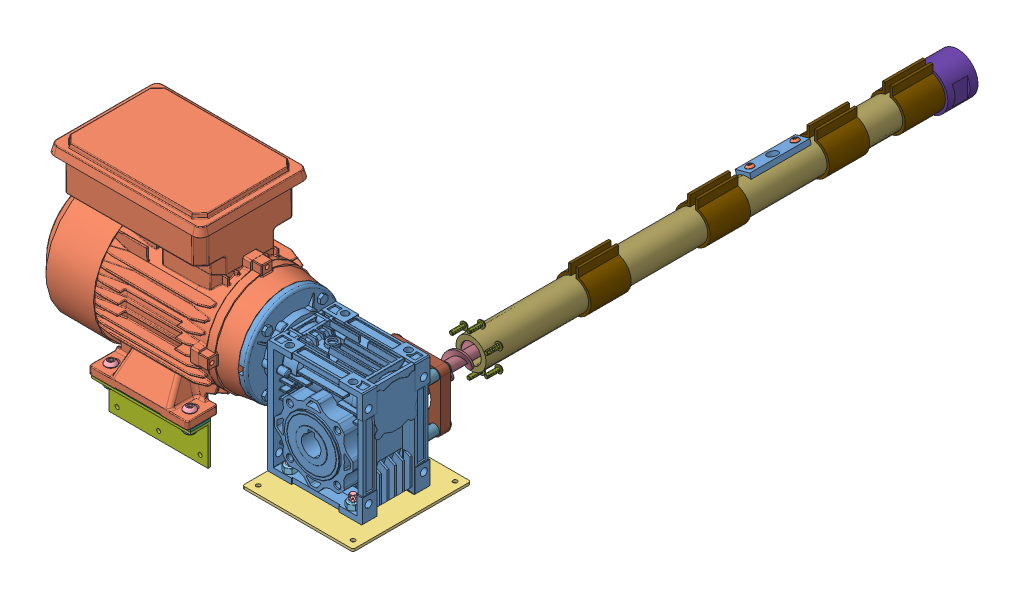
SolidWorks assembly coplete extruder assembly, configuration Default. Lengths in mm.
Overall size (405 416.05 925.2).
61 component instances, 24 part files, 64 mates.
Components (placement in the parent):
- motor assembly-1: motor assembly [Default] at (94.2301 96.5097 233.5212) size (405 416.05 596.46)
  - Redüktör Limöz LRP 50 1e25-1: Redüktör Limöz LRP 50 1e25 [Varsayılan] at (76.2256 70.7411 124.7447) size (140 170.5 120)
  - Gamak 0.75 KW Monofeze Motor-1: Gamak 0.75 KW Monofeze Motor [Varsayılan] at (-3.7744 121.2411 124.7447) x (0 0 1) z (-1 0 0) size (161.7 221.7 280.5)
  - gearbox plate-2: gearbox plate [Default] at (86.2256 7.5661 124.7447) x (0 0 -1) z (1 0 0) size (149 3.17 140)
  - 91239A427_CLASS 10.9 STL BUTTON-HEAD SOCKET CAP SCREW-1: 91239A427_CLASS 10.9 STL BUTTON-HEAD SOCKET CAP SCREW [91239A427] at (36.7256 3.1661 159.7447) x (1 0 0) z (0 -1 0) size (14 14 30.18)
  - 91239A427_CLASS 10.9 STL BUTTON-HEAD SOCKET CAP SCREW-2: 91239A427_CLASS 10.9 STL BUTTON-HEAD SOCKET CAP SCREW [91239A427] at (36.7256 3.1661 89.7447) x (1 0 0) z (0 -1 0) size (14 14 30.18)
  - 91239A427_CLASS 10.9 STL BUTTON-HEAD SOCKET CAP SCREW-3: 91239A427_CLASS 10.9 STL BUTTON-HEAD SOCKET CAP SCREW [91239A427] at (116.7256 3.1661 89.7447) x (1 0 0) z (0 -1 0) size (14 14 30.18)
  - 91239A427_CLASS 10.9 STL BUTTON-HEAD SOCKET CAP SCREW-4: 91239A427_CLASS 10.9 STL BUTTON-HEAD SOCKET CAP SCREW [91239A427] at (116.7256 3.1661 159.7447) x (1 0 0) z (0 -1 0) size (14 14 30.18)
  - 94645A210_ZINC-PLATED CLASS 10 STL NYLON-INSERT LOCKNUT-1: 94645A210_ZINC-PLATED CLASS 10 STL NYLON-INSERT LOCKNUT [94645A210] at (36.7256 17.7411 159.7447) size (13 8.23 15.01)
  - 94645A210_ZINC-PLATED CLASS 10 STL NYLON-INSERT LOCKNUT-2: 94645A210_ZINC-PLATED CLASS 10 STL NYLON-INSERT LOCKNUT [94645A210] at (116.7256 17.7411 159.7447) size (13 8.23 15.01)
  - 94645A210_ZINC-PLATED CLASS 10 STL NYLON-INSERT LOCKNUT-3: 94645A210_ZINC-PLATED CLASS 10 STL NYLON-INSERT LOCKNUT [94645A210] at (116.7256 17.7411 89.7447) size (13 8.23 15.01)
  - 94645A210_ZINC-PLATED CLASS 10 STL NYLON-INSERT LOCKNUT-4: 94645A210_ZINC-PLATED CLASS 10 STL NYLON-INSERT LOCKNUT [94645A210] at (36.7256 17.7411 89.7447) size (13 8.23 15.01)
  - 91239A427_CLASS 10.9 STL BUTTON-HEAD SOCKET CAP SCREW-5: 91239A427_CLASS 10.9 STL BUTTON-HEAD SOCKET CAP SCREW [91239A427] at (-159.7744 55.6411 189.7447) x (1 0 0) z (0 1 0) size (14 14 30.18)
  - 91239A427_CLASS 10.9 STL BUTTON-HEAD SOCKET CAP SCREW-6: 91239A427_CLASS 10.9 STL BUTTON-HEAD SOCKET CAP SCREW [91239A427] at (-59.7744 55.6411 189.7447) x (1 0 0) z (0 1 0) size (14 14 30.18)
  - 91239A427_CLASS 10.9 STL BUTTON-HEAD SOCKET CAP SCREW-7: 91239A427_CLASS 10.9 STL BUTTON-HEAD SOCKET CAP SCREW [91239A427] at (-159.7744 55.6411 59.6704) x (1 0 0) z (0 1 0) size (14 14 30.18)
  - 91239A427_CLASS 10.9 STL BUTTON-HEAD SOCKET CAP SCREW-8: 91239A427_CLASS 10.9 STL BUTTON-HEAD SOCKET CAP SCREW [91239A427] at (-59.7744 55.6411 59.7447) x (1 0 0) z (0 1 0) size (14 14 30.18)
  - motor dampener-1: motor dampener [Default] at (-109.7744 38.3661 188.7697) size (125 2.88 25.4)
  - motor mount-1: motor mount [Default] at (-172.2744 -12.4339 176.0697) x (0 0 -1) z (1 0 0) size (25.4 50.8 125)
  - motor mount-2: motor mount [Default] at (-47.2744 -12.4339 73.3454) x (0 0 1) z (-1 0 0) size (25.4 50.8 125)
  - motor dampener-3: motor dampener [Default] at (-109.7744 38.3661 60.6454) x (-1 0 0) z (0 0 -1) size (125 2.88 25.4)
  - 94645A210_ZINC-PLATED CLASS 10 STL NYLON-INSERT LOCKNUT-5: 94645A210_ZINC-PLATED CLASS 10 STL NYLON-INSERT LOCKNUT [94645A210] at (-159.7744 35.1911 189.7447) x (-0.837169 0 -0.546944) z (-0.546944 0 0.837169) size (13 8.23 15.01)
  - 94645A210_ZINC-PLATED CLASS 10 STL NYLON-INSERT LOCKNUT-6: 94645A210_ZINC-PLATED CLASS 10 STL NYLON-INSERT LOCKNUT [94645A210] at (-59.7744 35.1911 189.7447) x (-0.837169 0 -0.546944) z (-0.546944 0 0.837169) size (13 8.23 15.01)
  - 94645A210_ZINC-PLATED CLASS 10 STL NYLON-INSERT LOCKNUT-7: 94645A210_ZINC-PLATED CLASS 10 STL NYLON-INSERT LOCKNUT [94645A210] at (-159.7744 35.1911 59.6704) x (-0.837169 0 -0.546944) z (-0.546944 0 0.837169) size (13 8.23 15.01)
  - 94645A210_ZINC-PLATED CLASS 10 STL NYLON-INSERT LOCKNUT-8: 94645A210_ZINC-PLATED CLASS 10 STL NYLON-INSERT LOCKNUT [94645A210] at (-59.7744 35.1911 59.6704) x (-0.837169 0 -0.546944) z (-0.546944 0 0.837169) size (13 8.23 15.01)
- motor keyed assembly-1: motor keyed assembly [Default] at (179.7303 160.2957 356.7051) x (-1 0 0) z (0 0 -1) size (38.35 38.35 70)
  - key-1: key [Default] at (9.2746 18.9552 8.4391) size (8 7 32)
  - motor adaptor-1: motor adaptor [Default] at (9.2746 6.9552 4.4391) size (31.75 31.75 70)
  - 92095A208_18-8 SS BUTTON-HEAD SOCKET CAP SCREW-1: 92095A208_18-8 SS BUTTON-HEAD SOCKET CAP SCREW [92095A208] at (9.2746 29.2556 61.7391) x (0.982212 0 -0.187776) z (0 1 0) size (9.5 9.5 13.21)
  - 92095A208_18-8 SS BUTTON-HEAD SOCKET CAP SCREW-2: 92095A208_18-8 SS BUTTON-HEAD SOCKET CAP SCREW [92095A208] at (31.575 6.9552 61.7391) x (0 -0.452478 -0.891775) z (1 0 0) size (9.5 9.5 13.21)
- hopper body-1: hopper body [Default] at (130.4149 128.2753 188.7593) size (75 75 12.7)
  - hopper body-1: hopper body [Default] at (40.0409 38.9756 14.8067) (suppressed, hidden)
  - thrust bearing plate-1: thrust bearing plate [Default] at (40.0409 38.9756 78.3067) size (75 75 12.7)
- barrel Assembly-1: barrel Assembly [Default] at (387.3105 -120.5193 393.6593) x (-1 0 0) z (0 0 -1) size (38.1 38.1 609.6)
  - barrel-1: barrel [Default] at (216.8548 287.7701 113.8933) size (38.1 38.1 609.6)
  - pelletizer plate mount-1: pelletizer plate mount [Default] at (216.8548 287.7701 190.0933) (suppressed, hidden)
- 2_1 compression degas screw-1: 2_1 compression degas screw [Default] at (170.4557 167.2509 -378.134) size (26.05 26.04 688.01)
- thrust bering plate stsandoff-1: thrust bering plate stsandoff [Default] at (140.4557 197.2509 279.766) size (12.7 12.7 35)
- thrust bering plate stsandoff-2: thrust bering plate stsandoff [Default] at (140.4557 137.2509 279.766) size (12.7 12.7 35)
- thrust bering plate stsandoff-3: thrust bering plate stsandoff [Default] at (200.4557 197.2509 279.766) size (12.7 12.7 35)
- thrust bering plate stsandoff-4: thrust bering plate stsandoff [Default] at (200.4557 137.2509 279.766) size (12.7 12.7 35)
- feed tube assembly-1: feed tube assembly [Default] at (151.3893 181.3032 202.7167)
  - hopper tube-1: hopper tube [Default] at (19.0664 1.1876 38.8858) (suppressed, hidden)
  - tube hopper base-1: tube hopper base [Default] at (19.0664 1.1876 38.8858) (suppressed, hidden)
- 92095A299_18-8 SS BUTTON-HEAD SOCKET CAP SCREW-1: 92095A299_18-8 SS BUTTON-HEAD SOCKET CAP SCREW [92095A299] at (200.4557 197.2509 262.666) x (-0.923728 -0.383049 0) z (0 0 -1) size (14 14 60.2)
- 92095A299_18-8 SS BUTTON-HEAD SOCKET CAP SCREW-2: 92095A299_18-8 SS BUTTON-HEAD SOCKET CAP SCREW [92095A299] at (140.4557 197.2509 262.666) x (-0.923728 -0.383049 0) z (0 0 -1) size (14 14 60.2)
- 92095A299_18-8 SS BUTTON-HEAD SOCKET CAP SCREW-3: 92095A299_18-8 SS BUTTON-HEAD SOCKET CAP SCREW [92095A299] at (140.4557 137.2509 262.666) x (-0.923728 -0.383049 0) z (0 0 -1) size (14 14 60.2)
- 92095A299_18-8 SS BUTTON-HEAD SOCKET CAP SCREW-4: 92095A299_18-8 SS BUTTON-HEAD SOCKET CAP SCREW [92095A299] at (200.4557 137.2509 262.666) x (-0.923728 -0.383049 0) z (0 0 -1) size (14 14 60.2)
- 92095A212_18-8 SS BUTTON-HEAD SOCKET CAP SCREW-1: 92095A212_18-8 SS BUTTON-HEAD SOCKET CAP SCREW [92095A212] at (170.4557 141.8509 188.116) x (-0.923728 -0.383049 0) z (0 0 -1) size (9.5 9.5 19.24)
- 92095A212_18-8 SS BUTTON-HEAD SOCKET CAP SCREW-2: 92095A212_18-8 SS BUTTON-HEAD SOCKET CAP SCREW [92095A212] at (192.4528 154.5509 188.116) x (-0.923728 -0.383049 0) z (0 0 -1) size (9.5 9.5 19.24)
- 92095A212_18-8 SS BUTTON-HEAD SOCKET CAP SCREW-3: 92095A212_18-8 SS BUTTON-HEAD SOCKET CAP SCREW [92095A212] at (192.4528 179.9509 188.116) x (-0.923728 -0.383049 0) z (0 0 -1) size (9.5 9.5 19.24)
- 92095A212_18-8 SS BUTTON-HEAD SOCKET CAP SCREW-4: 92095A212_18-8 SS BUTTON-HEAD SOCKET CAP SCREW [92095A212] at (170.4557 192.6509 188.116) x (-0.923728 -0.383049 0) z (0 0 -1) size (9.5 9.5 19.24)
- 92095A212_18-8 SS BUTTON-HEAD SOCKET CAP SCREW-5: 92095A212_18-8 SS BUTTON-HEAD SOCKET CAP SCREW [92095A212] at (148.4587 179.9509 188.116) x (-0.923728 -0.383049 0) z (0 0 -1) size (9.5 9.5 19.24)
- 92095A212_18-8 SS BUTTON-HEAD SOCKET CAP SCREW-6: 92095A212_18-8 SS BUTTON-HEAD SOCKET CAP SCREW [92095A212] at (148.4587 154.5509 188.116) x (-0.923728 -0.383049 0) z (0 0 -1) size (9.5 9.5 19.24)
- nozzle-1: nozzle [Default] at (170.4557 167.2509 -374.284) x (0 -1 0) z (0 0 -1) size (50.8 50.8 38.1)
- heater band standing-1: heater band standing [Default] at (170.4557 167.2509 -374.284) size (44.45 53.98 50.8)
- heater band standing-2: heater band standing [Default] at (170.4557 167.2509 -278.484) size (44.45 53.98 50.8)
- heater band standing-3: heater band standing [Default] at (170.4557 167.2509 -127.684) size (44.45 53.98 50.8)
- heater band standing-4: heater band standing [Default] at (170.4557 167.2509 23.116) size (44.45 53.98 50.8)
- degas body base-1: degas body base [Default] at (166.1826 183.1983 -183.784) x (0 0 -1) z (0.965926 0.258819 0) size (76.07 6.35 19)
- 91239A222_CLASS 10.9 STL BUTTON-HEAD SOCKET CAP SCREW-1: 91239A222_CLASS 10.9 STL BUTTON-HEAD SOCKET CAP SCREW [91239A222] at (163.8274 191.9882 -155.209) x (0.933013 0.25 0.258819) z (-0.258819 0.965926 0) size (9.5 9.5 11.19)
- 91239A222_CLASS 10.9 STL BUTTON-HEAD SOCKET CAP SCREW-2: 91239A222_CLASS 10.9 STL BUTTON-HEAD SOCKET CAP SCREW [91239A222] at (163.8274 191.9882 -212.359) x (0.933013 0.25 0.258819) z (-0.258819 0.965926 0) size (9.5 9.5 11.19)
Mates (geometry in assembly coordinates):
- Coincident1: coincident anti-aligned: plane of motor assembly-1/Redüktör Limöz LRP 50 1e25-1 through (170.4557 167.2509 312.266) normal (0 0 -1); plane of motor keyed assembly-1/motor adaptor-1 through (170.4557 167.2509 312.266) normal (0 0 1)
- Parallel1: parallel anti-aligned: plane of motor assembly-1/Redüktör Limöz LRP 50 1e25-1 through (174.4557 179.0936 288.766) normal (-1 0 0); plane of motor keyed assembly-1/key-1 through (174.4557 175.7509 316.266) normal (1 0 0)
- Concentric1: concentric aligned: cylinder of motor assembly-1/Redüktör Limöz LRP 50 1e25-1 through (170.4557 167.2509 288.766) axis (0 0 1) radius 12.5; cylinder of motor keyed assembly-1/motor adaptor-1 through (170.4557 167.2509 282.266) axis (0 0 1) radius 15.875
- Concentric2: concentric aligned: cylinder of motor keyed assembly-1/motor adaptor-1 through (170.4557 167.2509 307.666) axis (0 0 -1) radius 9.5504; cylinder of hopper body-1/hopper body-1 through (170.4557 167.2509 279.766) axis (0 0 -1) radius 12.7254
- Parallel2: parallel aligned: plane of motor assembly-1/gearbox plate-2 through (180.4557 107.2509 358.266) normal (0 1 0); plane of hopper body-1/hopper body-1 through (170.4557 182.4909 203.566) normal (0 1 0)
- Coincident4: coincident anti-aligned: plane of hopper body-1/hopper body-1 through (170.4557 167.2509 203.566) normal (0 0 -1); plane of barrel Assembly-1/pelletizer plate mount-1 through (170.4557 167.2509 203.566) normal (0 0 1)
- Concentric3: concentric aligned: cylinder of hopper body-1/hopper body-1 through (170.4557 192.6509 209.916) axis (0 0 -1) radius 2.665; cylinder of barrel Assembly-1/pelletizer plate mount-1 through (170.4557 192.6509 203.567) axis (0 0 -1) radius 2.665
- Concentric4: concentric anti-aligned: cylinder of hopper body-1/hopper body-1 through (170.4557 167.2509 216.266) axis (0 0 -1) radius 31.75; cylinder of barrel Assembly-1/pelletizer plate mount-1 through (170.4557 167.2509 190.866) axis (0 0 1) radius 31.75
- Concentric5: concentric aligned: cylinder of hopper body-1/hopper body-1 through (170.4557 167.2509 279.766) axis (0 0 -1) radius 12.7254; cylinder of 2_1 compression degas screw-1 through (170.4557 167.2509 282.266) axis (0 0 -1) radius 12.7
- Parallel3: parallel aligned: plane of motor keyed assembly-1/92095A208_18-8 SS BUTTON-HEAD SOCKET CAP SCREW-1 through (169.9863 189.5513 292.5105) normal (0 1 0); plane of 2_1 compression degas screw-1 through (170.4557 174.8709 288.616) normal (0 1 0)
- Coincident7: coincident anti-aligned: plane of motor assembly-1/Redüktör Limöz LRP 50 1e25-1 through (170.4557 167.2509 314.766) normal (0 0 -1); plane of thrust bering plate stsandoff-4 through (200.4557 137.2509 314.766) normal (0 0 1)
- Concentric6: concentric anti-aligned: cylinder of motor assembly-1/Redüktör Limöz LRP 50 1e25-1 through (200.4557 137.2509 314.766) axis (0 0 1) radius 3.5; cylinder of thrust bering plate stsandoff-4 through (200.4557 137.2509 314.766) axis (0 0 -1) radius 4.165
- Coincident8: coincident anti-aligned: plane of hopper body-1/thrust bearing plate-1 through (170.4557 167.2509 279.766) normal (0 0 1); plane of thrust bering plate stsandoff-4 through (200.4557 137.2509 279.766) normal (0 0 -1)
- Coincident9: coincident anti-aligned: circle of motor keyed assembly-1/motor adaptor-1; plane of 2_1 compression degas screw-1 through (170.4557 167.2509 307.666) normal (0 0 1)
- Coincident10: coincident anti-aligned: plane of motor assembly-1/Redüktör Limöz LRP 50 1e25-1 through (170.4557 167.2509 314.766) normal (0 0 -1); plane of thrust bering plate stsandoff-3 through (200.4557 197.2509 314.766) normal (0 0 1)
- Concentric7: concentric anti-aligned: cylinder of motor assembly-1/Redüktör Limöz LRP 50 1e25-1 through (200.4557 197.2509 314.766) axis (0 0 1) radius 3.5; cylinder of thrust bering plate stsandoff-3 through (200.4557 197.2509 314.766) axis (0 0 -1) radius 6.35
- Coincident11: coincident anti-aligned: plane of hopper body-1/thrust bearing plate-1 through (170.4557 167.2509 279.766) normal (0 0 1); plane of thrust bering plate stsandoff-1 through (140.4557 197.2509 279.766) normal (0 0 -1)
- Concentric8: concentric anti-aligned: cylinder of hopper body-1/thrust bearing plate-1 through (140.4557 197.2509 267.065) axis (0 0 1) radius 4.165; cylinder of thrust bering plate stsandoff-1 through (140.4557 197.2509 314.766) axis (0 0 -1) radius 6.35
- Coincident12: coincident anti-aligned: plane of hopper body-1/thrust bearing plate-1 through (170.4557 167.2509 279.766) normal (0 0 1); plane of thrust bering plate stsandoff-2 through (140.4557 137.2509 279.766) normal (0 0 -1)
- Concentric9: concentric anti-aligned: cylinder of hopper body-1/thrust bearing plate-1 through (140.4557 137.2509 267.065) axis (0 0 1) radius 4.165; cylinder of thrust bering plate stsandoff-2 through (140.4557 137.2509 314.766) axis (0 0 -1) radius 6.35
- Coincident13: coincident anti-aligned: plane of hopper body-1/hopper body-1 through (170.4557 182.4909 203.566) normal (0 1 0); plane of feed tube assembly-1/tube hopper base-1 through (170.4557 182.4909 241.6025) normal (0 -1 0)
- Concentric10: concentric aligned: cylinder of hopper body-1/hopper body-1 through (185.7757 176.1409 221.266) axis (0 1 0) radius 2.5; cylinder of feed tube assembly-1/tube hopper base-1 through (185.7757 182.4899 221.266) axis (0 1 0) radius 2.665
- Concentric11: concentric aligned: cylinder of hopper body-1/hopper body-1 through (155.1357 176.1409 221.266) axis (0 1 0) radius 2.5; cylinder of feed tube assembly-1/tube hopper base-1 through (155.1357 182.4899 221.266) axis (0 1 0) radius 2.665
- Coincident14: coincident anti-aligned: plane of hopper body-1/thrust bearing plate-1 through (170.4557 167.2509 267.066) normal (0 0 -1); plane of 92095A299_18-8 SS BUTTON-HEAD SOCKET CAP SCREW-4 through (203.1371 130.7848 267.066) normal (0 0 1)
- Concentric12: concentric anti-aligned: cylinder of hopper body-1/thrust bearing plate-1 through (200.4557 137.2509 267.065) axis (0 0 1) radius 4.165; cylinder of 92095A299_18-8 SS BUTTON-HEAD SOCKET CAP SCREW-4 through (200.4557 137.2509 262.666) axis (0 0 -1) radius 7
- Coincident15: coincident anti-aligned: plane of hopper body-1/thrust bearing plate-1 through (170.4557 167.2509 267.066) normal (0 0 -1); plane of 92095A299_18-8 SS BUTTON-HEAD SOCKET CAP SCREW-1 through (203.1371 190.7848 267.066) normal (0 0 1)
- Concentric13: concentric anti-aligned: cylinder of hopper body-1/thrust bearing plate-1 through (200.4557 197.2509 267.065) axis (0 0 1) radius 4.165; cylinder of 92095A299_18-8 SS BUTTON-HEAD SOCKET CAP SCREW-1 through (200.4557 197.2509 262.666) axis (0 0 -1) radius 7
- Coincident16: coincident anti-aligned: plane of hopper body-1/thrust bearing plate-1 through (170.4557 167.2509 267.066) normal (0 0 -1); plane of 92095A299_18-8 SS BUTTON-HEAD SOCKET CAP SCREW-2 through (143.1371 190.7848 267.066) normal (0 0 1)
- Concentric14: concentric anti-aligned: cylinder of hopper body-1/thrust bearing plate-1 through (140.4557 197.2509 267.065) axis (0 0 1) radius 4.165; cylinder of 92095A299_18-8 SS BUTTON-HEAD SOCKET CAP SCREW-2 through (140.4557 197.2509 262.666) axis (0 0 -1) radius 7
- Coincident17: coincident anti-aligned: plane of hopper body-1/thrust bearing plate-1 through (170.4557 167.2509 267.066) normal (0 0 -1); plane of 92095A299_18-8 SS BUTTON-HEAD SOCKET CAP SCREW-3 through (143.1371 130.7848 267.066) normal (0 0 1)
- Concentric15: concentric anti-aligned: cylinder of hopper body-1/thrust bearing plate-1 through (140.4557 137.2509 267.065) axis (0 0 1) radius 4.165; cylinder of 92095A299_18-8 SS BUTTON-HEAD SOCKET CAP SCREW-3 through (140.4557 137.2509 262.666) axis (0 0 -1) radius 7
- Coincident18: coincident anti-aligned: plane of barrel Assembly-1/pelletizer plate mount-1 through (170.4557 167.2509 190.866) normal (0 0 -1); plane of 92095A212_18-8 SS BUTTON-HEAD SOCKET CAP SCREW-1 through (172.2752 137.4632 190.866) normal (0 0 1)
- Concentric16: concentric aligned: cylinder of barrel Assembly-1/pelletizer plate mount-1 through (170.4557 141.8509 203.567) axis (0 0 -1) radius 2.665; circle of 92095A212_18-8 SS BUTTON-HEAD SOCKET CAP SCREW-1
- Coincident19: coincident anti-aligned: plane of barrel Assembly-1/pelletizer plate mount-1 through (170.4557 167.2509 190.866) normal (0 0 -1); plane of 92095A212_18-8 SS BUTTON-HEAD SOCKET CAP SCREW-2 through (194.2722 150.1632 190.866) normal (0 0 1)
- Concentric17: concentric aligned: cylinder of barrel Assembly-1/pelletizer plate mount-1 through (192.4528 154.5509 203.567) axis (0 0 -1) radius 2.665; cylinder of 92095A212_18-8 SS BUTTON-HEAD SOCKET CAP SCREW-2 through (192.4528 154.5509 188.116) axis (0 0 -1) radius 4.75
- Coincident20: coincident anti-aligned: plane of barrel Assembly-1/pelletizer plate mount-1 through (170.4557 167.2509 190.866) normal (0 0 -1); plane of 92095A212_18-8 SS BUTTON-HEAD SOCKET CAP SCREW-3 through (194.2722 175.5632 190.866) normal (0 0 1)
- Concentric18: concentric aligned: cylinder of barrel Assembly-1/pelletizer plate mount-1 through (192.4528 179.9509 203.567) axis (0 0 -1) radius 2.665; cylinder of 92095A212_18-8 SS BUTTON-HEAD SOCKET CAP SCREW-3 through (192.4528 179.9509 188.116) axis (0 0 -1) radius 4.75
- Coincident21: coincident anti-aligned: plane of barrel Assembly-1/pelletizer plate mount-1 through (170.4557 167.2509 190.866) normal (0 0 -1); plane of 92095A212_18-8 SS BUTTON-HEAD SOCKET CAP SCREW-4 through (172.2752 188.2632 190.866) normal (0 0 1)
- Concentric19: concentric aligned: cylinder of barrel Assembly-1/pelletizer plate mount-1 through (170.4557 192.6509 203.567) axis (0 0 -1) radius 2.665; cylinder of 92095A212_18-8 SS BUTTON-HEAD SOCKET CAP SCREW-4 through (170.4557 192.6509 188.116) axis (0 0 -1) radius 4.75
- Coincident22: coincident anti-aligned: plane of barrel Assembly-1/pelletizer plate mount-1 through (170.4557 167.2509 190.866) normal (0 0 -1); plane of 92095A212_18-8 SS BUTTON-HEAD SOCKET CAP SCREW-5 through (150.2782 175.5632 190.866) normal (0 0 1)
- Concentric20: concentric aligned: cylinder of barrel Assembly-1/pelletizer plate mount-1 through (148.4587 179.9509 203.567) axis (0 0 -1) radius 2.665; cylinder of 92095A212_18-8 SS BUTTON-HEAD SOCKET CAP SCREW-5 through (148.4587 179.9509 188.116) axis (0 0 -1) radius 4.75
- Coincident23: coincident anti-aligned: plane of barrel Assembly-1/pelletizer plate mount-1 through (170.4557 167.2509 190.866) normal (0 0 -1); plane of 92095A212_18-8 SS BUTTON-HEAD SOCKET CAP SCREW-6 through (150.2782 150.1632 190.866) normal (0 0 1)
- Concentric21: concentric aligned: cylinder of barrel Assembly-1/pelletizer plate mount-1 through (148.4587 154.5509 203.567) axis (0 0 -1) radius 2.665; cylinder of 92095A212_18-8 SS BUTTON-HEAD SOCKET CAP SCREW-6 through (148.4587 154.5509 188.116) axis (0 0 -1) radius 4.75
- Coincident24: coincident anti-aligned: plane of barrel Assembly-1/barrel-1 through (170.4557 167.2509 -406.034) normal (0 0 -1); plane of nozzle-1 through (170.4557 167.2509 -406.034) normal (0 0 1)
- Concentric23: concentric aligned: cylinder of barrel Assembly-1/barrel-1 through (170.4557 167.2509 -406.034) axis (0 0 1) radius 19.05; cylinder of nozzle-1 through (170.4557 167.2509 -412.384) axis (0 0 1) radius 25.4
- Concentric24: concentric anti-aligned: cylinder of barrel Assembly-1/barrel-1 through (170.4557 167.2509 -406.034) axis (0 0 1) radius 19.05; cylinder of heater band standing-1 through (170.4557 167.2509 -323.484) axis (0 0 -1) radius 19.05
- Coincident26: coincident anti-aligned: plane of nozzle-1 through (170.4557 167.2509 -374.284) normal (0 0 1); plane of heater band standing-1 through (170.4557 167.2509 -374.284) normal (0 0 -1)
- Parallel5: parallel aligned: plane of nozzle-1 through (192.5537 141.8499 -383.174) normal (1 0 0); plane of heater band standing-1 through (176.8057 199.0009 -323.484) normal (1 0 0)
- Concentric25: concentric anti-aligned: cylinder of barrel Assembly-1/barrel-1 through (170.4557 167.2509 -406.034) axis (0 0 1) radius 19.05; cylinder of heater band standing-2 through (170.4557 167.2509 -227.684) axis (0 0 -1) radius 19.05
- Coincident28: coincident aligned: plane of heater band standing-1 through (176.8057 199.0009 -323.484) normal (1 0 0); plane of heater band standing-2 through (176.8057 199.0009 -227.684) normal (1 0 0)
- Distance1: distance = 45 mm anti-aligned: plane of heater band standing-2 through (170.4557 167.2509 -278.484) normal (0 0 -1); plane of heater band standing-1 through (170.4557 167.2509 -323.484) normal (0 0 1)
- Concentric26: concentric anti-aligned: cylinder of barrel Assembly-1/barrel-1 through (170.4557 167.2509 -406.034) axis (0 0 1) radius 19.05; cylinder of heater band standing-3 through (170.4557 167.2509 -76.884) axis (0 0 -1) radius 19.05
- Distance2: distance = 100 mm anti-aligned: plane of heater band standing-3 through (170.4557 167.2509 -127.684) normal (0 0 -1); plane of heater band standing-2 through (170.4557 167.2509 -227.684) normal (0 0 1)
- Concentric27: concentric anti-aligned: cylinder of barrel Assembly-1/barrel-1 through (170.4557 167.2509 -406.034) axis (0 0 1) radius 19.05; cylinder of heater band standing-4 through (170.4557 167.2509 73.916) axis (0 0 -1) radius 19.05
- Coincident31: coincident aligned: plane of heater band standing-2 through (176.8057 199.0009 -227.684) normal (1 0 0); plane of heater band standing-3 through (176.8057 199.0009 -76.884) normal (1 0 0)
- Coincident32: coincident aligned: plane of heater band standing-3 through (176.8057 199.0009 -76.884) normal (1 0 0); plane of heater band standing-4 through (176.8057 199.0009 73.916) normal (1 0 0)
- Distance3: distance = 100 mm: line of heater band standing-4 through (173.6307 199.0009 23.116) axis (0 -1 0); plane of heater band standing-3 through (170.4557 167.2509 -76.884) normal (0 0 1)
- Coincident34: coincident anti-aligned: plane of barrel Assembly-1/barrel-1 through (166.1826 183.1983 279.766) normal (-0.258819 0.965926 0); plane of degas body base-1 through (166.1826 183.1983 -183.784) normal (0.258819 -0.965926 0)
- Concentric28: concentric aligned: cylinder of barrel Assembly-1/barrel-1 through (166.1826 183.1983 -155.209) axis (-0.258819 0.965926 0) radius 2.1; cylinder of degas body base-1 through (166.1829 183.1973 -155.209) axis (-0.258819 0.965926 0) radius 2.665
- Concentric29: concentric aligned: cylinder of barrel Assembly-1/barrel-1 through (166.1826 183.1983 -212.359) axis (-0.258819 0.965926 0) radius 2.1; cylinder of degas body base-1 through (166.1829 183.1973 -212.359) axis (-0.258819 0.965926 0) radius 2.665
- Coincident35: coincident anti-aligned: plane of degas body base-1 through (164.5391 189.3319 -183.784) normal (-0.258819 0.965926 0); plane of 91239A222_CLASS 10.9 STL BUTTON-HEAD SOCKET CAP SCREW-1 through (163.3516 189.0137 -150.6209) normal (0.258819 -0.965926 0)
- Concentric30: concentric aligned: cylinder of degas body base-1 through (166.1829 183.1973 -155.209) axis (-0.258819 0.965926 0) radius 2.665; cylinder of 91239A222_CLASS 10.9 STL BUTTON-HEAD SOCKET CAP SCREW-1 through (163.8274 191.9882 -155.209) axis (-0.258819 0.965926 0) radius 4.75
- Coincident36: coincident anti-aligned: plane of degas body base-1 through (164.5391 189.3319 -183.784) normal (-0.258819 0.965926 0); plane of 91239A222_CLASS 10.9 STL BUTTON-HEAD SOCKET CAP SCREW-2 through (163.3516 189.0137 -207.7709) normal (0.258819 -0.965926 0)
- Concentric31: concentric aligned: cylinder of degas body base-1 through (166.1829 183.1973 -212.359) axis (-0.258819 0.965926 0) radius 2.665; cylinder of 91239A222_CLASS 10.9 STL BUTTON-HEAD SOCKET CAP SCREW-2 through (163.8274 191.9882 -212.359) axis (-0.258819 0.965926 0) radius 4.75
